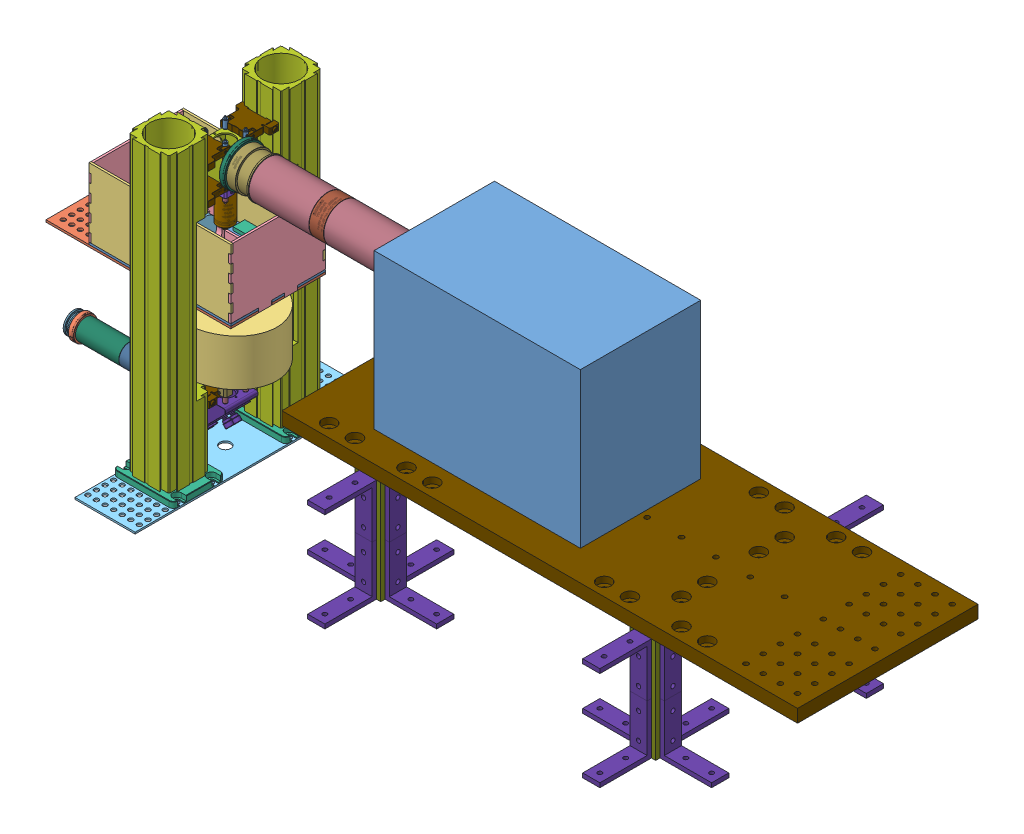
SolidWorks assembly Water Bath DRM, configuration Default. Lengths in mm.
Overall size (1204.68 450.6 419.1).
114 component instances, 38 part files, 41 mates.
Components (placement in the parent):
- WB_0p125_BaseThreaded-1: WB_0p125_BaseThreaded [Default] at (0 3.175 0) size (209.55 3.17 139.7)
- WB_0p125_Base-1: WB_0p125_Base [Default] at origin size (273.05 3.17 139.7)
- WB_0p125_Long-1: WB_0p125_Long [Default] at (0 57.15 -69.85) size (209.55 107.95 3.17)
- WB_0p125_Long-2: WB_0p125_Long [Default] at (0 57.15 66.675) size (209.55 107.95 3.17)
- WB_0p125_Short-1: WB_0p125_Short [Default] at (101.6 57.15 0) x (0 0 1) z (0 1 0) size (139.7 3.17 107.95)
- WB_0p125_Short-2: WB_0p125_Short [Default] at (-104.775 57.15 0) x (0 0 1) z (0 1 0) size (139.7 3.17 107.95)
- Table SubAssembly-1: Table SubAssembly [Default] at (-11.1846 -225.3996 0) x (0 0 -1) z (1 0 0) size (355.6 442.98 89.6)
  - Table-1: Table [Default] at origin size (355.6 2.54 88.9)
  - XT66P1-Solidworks-1: XT66P1-Solidworks [Default] at (-83.0224 2.286 37.592) x (-1 0 0) z (0 0 -1) size (76.2 8.89 89.28)
  - XT66P1-Solidworks-2: XT66P1-Solidworks [Default] at (83.0224 2.286 37.592) size (76.2 8.89 89.28)
  - KCB1-Solidworks-1: KCB1-Solidworks [Default] at (-24.13 99.7796 13.4747) x (0.000001 0 1) z (0 1 0) size (51.13 48.26 51.1) (hidden)
  - RCA1-Solidworks-1: RCA1-Solidworks [Default] at (-24.2926 205.6203 66.0649) x (0 0 -1) z (0 -1 0) size (56.5 73.55 8.89) (hidden)
  - RCA1-Solidworks-2: RCA1-Solidworks [Default] at (24.2926 108.2389 66.0649) x (0 0 -1) z (0 1 0) size (56.5 73.55 8.89) (hidden)
  - XT66-500-modified_v2-1: XT66-500-modified_v2 [Default] at (-83.0224 511.176 37.592) x (0 0 -1) z (0 -1 0) size (66.02 67.06 431.8)
  - XT66-500-modified_v2-2: XT66-500-modified_v2 [Default] at (83.0224 511.176 37.592) x (0 0 1) z (0 -1 0) size (66.02 67.06 431.8)
- Small Condenser Adjustable Sub-Assembly-1: Small Condenser Adjustable Sub-Assembly [Default] at (62.4754 -100.9396 20.3199) x (0 -1 0) z (0 0 1) size (204.14 301.96 127)
  - LB1437-Solidworks-1: LB1437-Solidworks [Default] at (76.2 -223.413 -20.3199) x (0.879994 0 -0.474985) z (0 -1 0) size (25.4 25.4 3.05)
  - LB1761-Solidworks-1: LB1761-Solidworks [Default] at (76.2 -78.613 -20.3199) x (0.962182 0 -0.272406) z (0 -1 0) size (25.4 25.4 8.98)
  - SM1L40-Solidworks-1: SM1L40-Solidworks [Default] at (78.3398 -122.5422 -22.1696) x (-0.992854 0 -0.119336) z (0 1 0) size (30.48 30.48 105.41)
  - CSA1003-Solidworks-1: CSA1003-Solidworks [Default] at (47.6181 -122.449 -34.035) x (0 -1 0) z (0 0 1) size (71.12 13.97 71.12)
  - LCP02-Solidworks-1: LCP02-Solidworks [Default] at (20.32 -35.5599 -20.32) x (0 0 -1) z (1 0 0) size (70.75 70.61 12.7)
  - ER1-Solidworks-1: ER1-Solidworks [Default] at (36.8841 -51.9737 -4.6825) x (0 -0.925141 -0.379624) z (0 -0.379624 0.925141) size (5.99 30.48 5.99)
  - ER1-Solidworks-3: ER1-Solidworks [Default] at (36.8841 -50.6608 -33.7724) x (0 -0.769482 0.638668) z (0 0.638668 0.769482) size (5.99 30.48 5.99)
  - ER1-Solidworks-4: ER1-Solidworks [Default] at (41.8559 -21.5595 -36.5057) x (0 -0.998351 -0.057413) z (0 0.057413 -0.998351) size (5.99 30.48 5.99)
  - SM1T2-Solidworks-1: SM1T2-Solidworks [Default] at (76.2 -248.6152 -20.3199) x (0.998592 0 -0.053039) z (0 1 0) size (31.75 31.75 12.7)
  - SM1L25-Solidworks-1: SM1L25-Solidworks [Default] at (139.9124 -186.275 -15.6668) x (0 -1 0) z (-0.806632 0 -0.591053) size (67.31 30.48 30.48)
  - CP08-Solidworks-3: CP08-Solidworks [Default] at (76.2 -69.215 -20.3199) x (0 0 -1) z (0 1 0) size (41.5 40.64 8.89)
  - KCB1-Solidworks-2: KCB1-Solidworks [Default] at (100.33 -11.43 3.8101) x (-1 0 0) z (0 -1 0) size (51.13 48.26 51.1)
  - ER1-Solidworks-6: ER1-Solidworks [Default] at (36.8841 -20.7263 -3.7781) x (0 -0.795862 0.605478) z (0 0.605478 0.795862) size (5.99 30.48 5.99)
  - RCA2-Solidworks-1: RCA2-Solidworks [Default] at (68.2294 -49.0321 -29.2771) x (0 1 0) z (-1 0 0) size (56.73 41.06 8.89)
  - RCA2-Solidworks-2: RCA2-Solidworks [Default] at (68.2294 -22.0879 -11.3628) x (0 -1 0) z (-1 0 0) size (56.73 41.06 8.89)
  - ER05-Solidworks-1: ER05-Solidworks [Default] at (92.6015 -68.5259 -5.9839) x (0.310188 0 -0.950675) z (0.950675 0 0.310188) size (5.99 17.78 5.99)
  - ER05-Solidworks-2: ER05-Solidworks [Default] at (59.8613 -68.5259 -4.5371) x (-0.22668 0 0.973969) z (-0.973969 0 -0.22668) size (5.99 17.78 5.99)
  - ER05-Solidworks-3: ER05-Solidworks [Default] at (92.2659 -68.5259 -34.1935) size (5.99 17.78 5.99)
  - ER05-Solidworks-4: ER05-Solidworks [Default] at (59.7556 -68.5259 -34.7555) x (-0.375833 0 0.926687) z (-0.926687 0 -0.375833) size (5.99 17.78 5.99)
  - SM1D12D-Solidworks-1: SM1D12D-Solidworks [Default] at (81.3975 -244.783 -22.8892) x (0.973299 0 -0.22954) z (0 1 0) size (35.81 35.81 11.94)
  - SM1D12D-Solidworks-2: SM1D12D-Solidworks [Default] at (70.9424 -73.1298 -22.7639) x (-0.788375 0 -0.615195) z (0 1 0) size (35.81 35.81 11.94)
  - ER1-Solidworks-9: ER1-Solidworks [Default] at (15.1859 -4.2179 -49.5429) x (0 0.95877 -0.284182) z (0 0.284182 0.95877) size (5.99 30.48 5.99)
  - ER1-Solidworks-10: ER1-Solidworks [Default] at (15.1859 -64.6339 -49.076) x (0 0.993069 0.117534) z (0 -0.117534 0.993069) size (5.99 30.48 5.99)
  - ER1-Solidworks-11: ER1-Solidworks [Default] at (15.1859 -4.6008 10.8986) x (0 0.995869 0.090807) z (0 -0.090807 0.995869) size (5.99 30.48 5.99)
  - ER1-Solidworks-12: ER1-Solidworks [Default] at (15.1859 -64.2349 10.4858) x (0 0.96466 -0.263499) z (0 0.263499 0.96466) size (5.99 30.48 5.99)
  - OlympusCondenser-1: OlympusCondenser [Default] at (7.0104 -35.56 -20.3199) x (0 -1 0) z (0 0 -1) size (152.4 107.95 127)
- 500 kHz Tank (21) Opticell-1: 500 kHz Tank (21) Opticell [Default] at (6.35 57.15 0) size (152.4 50.8 50.8)
- 500kHz-1: 500kHz [Default] at (-42.5918 31.75 0) x (1 0 0) z (0 -0.094104 0.995562) size (70.95 43.18 43.18)
- Opticell_Truncated-1: Opticell_Truncated [Default] at (22.5976 32.0671 2.9503) size (53.01 12.75 129.72)
- Objective Sub-Assembly-1: Objective Sub-Assembly [Default] at (61.6077 -289.593 114.3819) x (0 0 -1) z (0 -1 0) size (106.71 57.63 128.02)
  - CM1-DCH-Solidworks-1: CM1-DCH-Solidworks [Web Assembly] at (114.3818 -34.6924 -438.5894) x (0 -1 0) z (0 0 1) size (38.1 45.72 38.1)
  - CP16-Solidworks-1: CP16-Solidworks [Default] at (116.5677 -16.5858 -398.1348) x (0 -1 0) z (0 0 1) size (41.22 40.64 8.89)
  - RCA2-Solidworks-1: RCA2-Solidworks [Default] at (123.339 -21.2203 -499.1988) x (0 -1 0) z (0 0 1) size (56.73 41.06 8.89)
  - RCA2-Solidworks-2: RCA2-Solidworks [Default] at (105.4247 -48.1644 -499.1988) x (0 1 0) z (0 0 1) size (56.73 41.06 8.89)
  - N40X-NIR-Solidworks-1: N40X-NIR-Solidworks [Default] at (114.3819 -34.6923 -375.0894) x (0 0 1) z (0.875921 0.482454 0) size (61.98 27.94 27.94)
  - RCA2-Solidworks-3: RCA2-Solidworks [Default] at (105.4247 -48.1644 -452.2088) x (0 1 0) z (0 0 1) size (56.73 41.06 8.89)
  - RCA2-Solidworks-4: RCA2-Solidworks [Default] at (123.339 -21.2203 -452.2088) x (0 -1 0) z (0 0 1) size (56.73 41.06 8.89)
  - ER1-Solidworks-1: ER1-Solidworks [Default] at (100.293 -20.9473 -404.3535) x (-0.183947 -0.982936 0) z (0.982936 -0.183947 0) size (5.99 30.48 5.99)
  - ER1-Solidworks-2: ER1-Solidworks [Default] at (130.5299 -50.7349 -404.3535) x (0.020475 -0.99979 0) z (0.99979 0.020475 0) size (5.99 30.48 5.99)
  - ER1-Solidworks-3: ER1-Solidworks [Default] at (100.0093 -51.1105 -404.3535) x (-0.386185 -0.922421 0) z (0.922421 -0.386185 0) size (5.99 30.48 5.99)
  - ER1-Solidworks-4: ER1-Solidworks [Default] at (129.6817 -21.2139 -404.3535) x (-0.579753 -0.814792 0) z (0.814792 -0.579753 0) size (5.99 30.48 5.99)
  - ER05-Solidworks-1: ER05-Solidworks [Default] at (129.9725 -48.2584 -461.5035) x (0.933397 0.358845 0) z (-0.358845 0.933397 0) size (5.99 17.78 5.99)
  - ER05-Solidworks-2: ER05-Solidworks [Default] at (97.9162 -50.199 -461.5035) x (-0.886919 0.461926 0) z (-0.461926 -0.886919 0) size (5.99 17.78 5.99)
  - ER05-Solidworks-3: ER05-Solidworks [Default] at (128.9134 -21.1707 -461.5035) x (-0.900043 -0.4358 0) z (0.4358 -0.900043 0) size (5.99 17.78 5.99)
  - ER05-Solidworks-4: ER05-Solidworks [Default] at (100.2773 -18.4261 -461.5035) x (0.989892 0.141823 0) z (-0.141823 0.989892 0) size (5.99 17.78 5.99)
- Camera Sub-Assembly-1: Camera Sub-Assembly [Default] at (36.8213 148.9964 0) x (0 -0.692092 0.721809) z (-1 0 0) size (71.93 71.93 298.88)
  - SM2NFM2-Solidworks-1: SM2NFM2-Solidworks [Default] at (0 0 -285.6832) x (0 1 0) z (-1 0 0) size (63.5 16.37 63.5)
  - TTL200-S8-Solidworks-1: TTL200-S8-Solidworks [Default] at (0 0 -152.5317) size (55.88 55.88 28)
  - SM2V15-Solidworks-1: SM2V15-Solidworks [Default] at (18.0496 -29.8565 -288.422) x (0 0 -1) z (0.951776 0.306793 0) size (51.56 57.15 57.15)
  - SM2M35-Solidworks-1: SM2M35-Solidworks [Default] at (-10.7846 9.351 -219.5042) x (0.99081 -0.135264 0) z (0 0 1) size (55.88 55.88 88.9)
  - SM2M35-Solidworks-2: SM2M35-Solidworks [Default] at (-11.8362 7.9783 -108.9542) x (0.999895 -0.014459 0) z (0 0 1) size (55.88 55.88 88.9)
  - SM2V15-Solidworks-2: SM2V15-Solidworks [Default] at (-9.1968 -33.7176 -16.6413) x (0 0 1) z (-0.999373 0.035397 0) size (51.56 57.15 57.15)
  - SM1T2-Solidworks-1: SM1T2-Solidworks [Default] at (0 0 1.778) x (0.997143 -0.075539 0) z (0 0 1) size (31.75 31.75 12.7)
  - SM2A6-Solidworks-2: SM2A6-Solidworks [Default] at (0 0 -9.144) size (51.69 51.69 5.08)
  - SM2D25D-Solidworks-1: SM2D25D-Solidworks [Default] at (-6.3593 1.1475 -12.9462) x (-1 0 0) z (0 0 -1) size (60.96 60.96 12.32)
- Full Assembly Total Support-1: Full Assembly Total Support [Default] at (624.8382 -22.4536 0) size (762 171.45 419.1)
  - Post SubAssembly-1: Post SubAssembly [Default] at (-254 -152.4 114.3) size (190.5 152.4 190.5)
    - Post-1: Post [Default] at origin size (38.1 152.4 38.1)
    - Hinge-1: Hinge [Default] at (-25.4 6.35 0) x (0 0 -1) z (0 -1 0) size (25.4 76.2 76.2)
    - Hinge-2: Hinge [Default] at (0 6.35 25.4) x (-1 0 0) z (0 -1 0) size (25.4 76.2 76.2)
    - Hinge-3: Hinge [Default] at (25.4 6.35 0) x (0 0 1) z (0 -1 0) size (25.4 76.2 76.2)
    - Hinge-4: Hinge [Default] at (0 6.35 -25.4) x (1 0 0) z (0 -1 0) size (25.4 76.2 76.2)
    - Hinge-5: Hinge [Default] at (25.4 146.05 0) x (0 0 1) z (-1 0 0) size (25.4 76.2 76.2)
    - Hinge-7: Hinge [Default] at (-25.4 146.05 0) x (0 0 -1) z (1 0 0) size (25.4 76.2 76.2)
    - Hinge-8: Hinge [Default] at (0 146.05 25.4) x (-1 0 0) z (0 0 -1) size (25.4 76.2 76.2)
    - Hinge-9: Hinge [Default] at (0 146.05 -25.4) size (25.4 76.2 76.2)
  - Post SubAssembly-2: Post SubAssembly [Default] at (-254 -152.4 -114.3) size (190.5 152.4 190.5)
    - Post-1: Post [Default] at origin size (38.1 152.4 38.1)
    - Hinge-1: Hinge [Default] at (-25.4 6.35 0) x (0 0 -1) z (0 -1 0) size (25.4 76.2 76.2)
    - Hinge-2: Hinge [Default] at (0 6.35 25.4) x (-1 0 0) z (0 -1 0) size (25.4 76.2 76.2)
    - Hinge-3: Hinge [Default] at (25.4 6.35 0) x (0 0 1) z (0 -1 0) size (25.4 76.2 76.2)
    - Hinge-4: Hinge [Default] at (0 6.35 -25.4) x (1 0 0) z (0 -1 0) size (25.4 76.2 76.2)
    - Hinge-5: Hinge [Default] at (25.4 146.05 0) x (0 0 1) z (-1 0 0) size (25.4 76.2 76.2)
    - Hinge-7: Hinge [Default] at (-25.4 146.05 0) x (0 0 -1) z (1 0 0) size (25.4 76.2 76.2)
    - Hinge-8: Hinge [Default] at (0 146.05 25.4) x (-1 0 0) z (0 0 -1) size (25.4 76.2 76.2)
    - Hinge-9: Hinge [Default] at (0 146.05 -25.4) size (25.4 76.2 76.2)
  - Post SubAssembly-3: Post SubAssembly [Default] at (152.4 -152.4 114.3) size (190.5 152.4 190.5)
    - Post-1: Post [Default] at origin size (38.1 152.4 38.1)
    - Hinge-1: Hinge [Default] at (-25.4 6.35 0) x (0 0 -1) z (0 -1 0) size (25.4 76.2 76.2)
    - Hinge-2: Hinge [Default] at (0 6.35 25.4) x (-1 0 0) z (0 -1 0) size (25.4 76.2 76.2)
    - Hinge-3: Hinge [Default] at (25.4 6.35 0) x (0 0 1) z (0 -1 0) size (25.4 76.2 76.2)
    - Hinge-4: Hinge [Default] at (0 6.35 -25.4) x (1 0 0) z (0 -1 0) size (25.4 76.2 76.2)
    - Hinge-5: Hinge [Default] at (25.4 146.05 0) x (0 0 1) z (-1 0 0) size (25.4 76.2 76.2)
    - Hinge-7: Hinge [Default] at (-25.4 146.05 0) x (0 0 -1) z (1 0 0) size (25.4 76.2 76.2)
    - Hinge-8: Hinge [Default] at (0 146.05 25.4) x (-1 0 0) z (0 0 -1) size (25.4 76.2 76.2)
    - Hinge-9: Hinge [Default] at (0 146.05 -25.4) size (25.4 76.2 76.2)
  - Post SubAssembly-4: Post SubAssembly [Default] at (152.4 -152.4 -114.3) size (190.5 152.4 190.5)
    - Post-1: Post [Default] at origin size (38.1 152.4 38.1)
    - Hinge-1: Hinge [Default] at (-25.4 6.35 0) x (0 0 -1) z (0 -1 0) size (25.4 76.2 76.2)
    - Hinge-2: Hinge [Default] at (0 6.35 25.4) x (-1 0 0) z (0 -1 0) size (25.4 76.2 76.2)
    - Hinge-3: Hinge [Default] at (25.4 6.35 0) x (0 0 1) z (0 -1 0) size (25.4 76.2 76.2)
    - Hinge-4: Hinge [Default] at (0 6.35 -25.4) x (1 0 0) z (0 -1 0) size (25.4 76.2 76.2)
    - Hinge-5: Hinge [Default] at (25.4 146.05 0) x (0 0 1) z (-1 0 0) size (25.4 76.2 76.2)
    - Hinge-7: Hinge [Default] at (-25.4 146.05 0) x (0 0 -1) z (1 0 0) size (25.4 76.2 76.2)
    - Hinge-8: Hinge [Default] at (0 146.05 25.4) x (-1 0 0) z (0 0 -1) size (25.4 76.2 76.2)
    - Hinge-9: Hinge [Default] at (0 146.05 -25.4) size (25.4 76.2 76.2)
  - Camera Shelf Full Support v2-1: Camera Shelf Full Support v2 [Default] at origin size (762 19.05 266.7)
- hpvx2-1: hpvx2 [Default] at (488.0998 -3.4036 0) size (311.15 228.6 177.8)
Mates (geometry in assembly coordinates):
- Coincident1: coincident aligned: plane of WB_0p125_BaseThreaded-1 through (-101.6 6.35 66.675) normal (0 0 1); plane of WB_0p125_Base-1 through (-101.6 3.175 66.675) normal (0 0 1)
- Coincident2: coincident aligned: plane of WB_0p125_BaseThreaded-1 through (101.6 6.35 66.675) normal (1 0 0); plane of WB_0p125_Base-1 through (101.6 3.175 66.675) normal (1 0 0)
- Coincident3: coincident anti-aligned: plane of WB_0p125_BaseThreaded-1 through (0 3.175 0) normal (0 -1 0); plane of WB_0p125_Base-1 through (0 3.175 0) normal (0 1 0)
- Coincident4: coordinate: point of WB_0p125_Base-1; point of assembly
- Coincident5: coincident aligned: plane of WB_0p125_BaseThreaded-1 through (101.6 6.35 66.675) normal (1 0 0); plane of WB_0p125_Long-2 through (101.6 6.35 69.85) normal (1 0 0)
- Coincident6: coincident anti-aligned: plane of WB_0p125_BaseThreaded-1 through (0 6.35 0) normal (0 1 0); plane of WB_0p125_Long-2 through (-101.6 6.35 69.85) normal (0 -1 0)
- Coincident8: coincident anti-aligned: plane of WB_0p125_BaseThreaded-1 through (0 6.35 0) normal (0 1 0); plane of WB_0p125_Long-1 through (-101.6 6.35 -66.675) normal (0 -1 0)
- Coincident9: coincident aligned: plane of WB_0p125_BaseThreaded-1 through (-101.6 6.35 66.675) normal (-1 0 0); plane of WB_0p125_Long-1 through (-101.6 6.35 -66.675) normal (-1 0 0)
- Coincident11: coincident anti-aligned: plane of WB_0p125_BaseThreaded-1 through (-101.6 6.35 66.675) normal (-1 0 0); plane of WB_0p125_Short-2 through (-101.6 57.15 0) normal (1 0 0)
- Coincident12: coincident anti-aligned: plane of WB_0p125_BaseThreaded-1 through (0 6.35 0) normal (0 1 0); plane of WB_0p125_Short-2 through (-101.6 6.35 -66.675) normal (0 -1 0)
- Coincident14: coincident anti-aligned: plane of WB_0p125_Long-2 through (0 57.15 66.675) normal (0 0 -1); plane of WB_0p125_Short-2 through (-101.6 107.95 66.675) normal (0 0 1)
- Coincident16: coincident anti-aligned: plane of WB_0p125_Long-2 through (0 57.15 66.675) normal (0 0 -1); plane of WB_0p125_Short-1 through (104.775 107.95 66.675) normal (0 0 1)
- Coincident18: coincident anti-aligned: plane of WB_0p125_Long-1 through (0 57.15 -66.675) normal (0 0 1); plane of WB_0p125_Short-2 through (-101.6 107.95 -66.675) normal (0 0 -1)
- Coincident19: coincident anti-aligned: plane of WB_0p125_BaseThreaded-1 through (-101.6 6.35 -66.675) normal (0 0 -1); plane of WB_0p125_Long-1 through (0 57.15 -66.675) normal (0 0 1)
- Coincident20: coincident aligned: plane of WB_0p125_Long-2 through (104.775 107.95 66.675) normal (1 0 0); plane of WB_0p125_Short-1 through (104.775 57.15 0) normal (1 0 0)
- Coincident21: coincident aligned: plane of WB_0p125_Base-1 through (0 0 0) normal (0 -1 0); plane of WB_0p125_Short-1 through (104.775 0 9.525) normal (0 -1 0)
- Coincident28: coincident anti-aligned: plane of Table SubAssembly-1/Table-1 through (-11.1846 -225.3996 0) normal (0 0 -1); plane of assembly through (0 0 0) normal (0 0 1)
- Concentric7: concentric aligned: circle of Table SubAssembly-1/Table-1; circle of Small Condenser Adjustable Sub-Assembly-1/OlympusCondenser-1
- Parallel1: parallel aligned: plane of Table SubAssembly-1/XT66-500-modified_v2-1 through (6.0694 -214.2236 116.5515) normal (0 0 1); plane of Small Condenser Adjustable Sub-Assembly-1/CSA1003-Solidworks-1 through (62.4754 -100.9396 35.56) normal (0 0 1)
- Concentric8: concentric aligned: circle of WB_0p125_BaseThreaded-1; circle of 500 kHz Tank (21) Opticell-1
- Concentric10: concentric aligned: circle of WB_0p125_BaseThreaded-1; circle of 500 kHz Tank (21) Opticell-1
- Coincident29: coincident anti-aligned: plane of WB_0p125_BaseThreaded-1 through (0 6.35 0) normal (0 1 0); plane of 500 kHz Tank (21) Opticell-1 through (-69.85 6.35 25.4) normal (0 -1 0)
- Concentric11: concentric aligned: cylinder of 500 kHz Tank (21) Opticell-1 through (-146.1329 31.75 0) axis (-1 0 0) radius 22.225; cylinder of 500kHz-1 through (-42.5918 31.75 0) axis (-1 0 0) radius 21.59
- Coincident30: coincident anti-aligned: plane of 500 kHz Tank (21) Opticell-1 through (-4.9109 53.975 0) normal (-1 0 0); plane of 500kHz-1 through (-4.9109 53.2442 2.0317) normal (1 0 0)
- Coincident31: coincident anti-aligned: plane of 500 kHz Tank (21) Opticell-1 through (6.35 25.6921 0) normal (0 1 0); plane of Opticell_Truncated-1 through (22.5976 25.6921 2.9503) normal (0 -1 0)
- Coincident32: coincident anti-aligned: plane of 500 kHz Tank (21) Opticell-1 through (58.6526 25.6921 -25.4) normal (-1 0 0); plane of Opticell_Truncated-1 through (58.6526 34.5671 51.6503) normal (1 0 0)
- Coincident33: coincident anti-aligned: plane of WB_0p125_Base-1 through (0 0 0) normal (0 -1 0); plane of Small Condenser Adjustable Sub-Assembly-1/OlympusCondenser-1 through (26.9154 0 0) normal (0 1 0)
- Distance1: distance = 25.4 mm anti-aligned: plane of Small Condenser Adjustable Sub-Assembly-1/CP08-Solidworks-3 through (-2.2946 -197.4596 18.034) normal (0 -1 0); plane of Table SubAssembly-1/Table-1 through (-11.1846 -222.8596 0) normal (0 1 0)
- Concentric12: concentric aligned: circle of Table SubAssembly-1/Table-1; circle of Objective Sub-Assembly-1/N40X-NIR-Solidworks-1
- Parallel2: parallel aligned: plane of Table SubAssembly-1/XT66-500-modified_v2-2 through (59.4152 -214.2236 -103.3604) normal (1 0 0); plane of Objective Sub-Assembly-1/CM1-DCH-Solidworks-1 through (45.9653 129.9464 -19.05) normal (1 0 0)
- Concentric13: concentric aligned: circle of Objective Sub-Assembly-1/CM1-DCH-Solidworks-1; cylinder of Camera Sub-Assembly-1/SM2M35-Solidworks-2 through (136.618 148.9964 0) axis (-1 0 0) radius 27.94
- Distance2: distance = 40.64 mm aligned: plane of Table SubAssembly-1/XT66-500-modified_v2-2 through (-6.6004 217.5764 -49.4934) normal (0 1 0); plane of Objective Sub-Assembly-1/RCA2-Solidworks-1 through (45.9653 176.9364 -13.6187) normal (0 1 0)
- Coincident36: coincident anti-aligned: plane of Objective Sub-Assembly-1/CM1-DCH-Solidworks-1 through (45.9653 129.9464 -19.05) normal (1 0 0); plane of Camera Sub-Assembly-1/SM2A6-Solidworks-2 through (45.9653 158.4842 9.0972) normal (-1 0 0)
- Concentric14: concentric anti-aligned: cylinder of Camera Sub-Assembly-1/SM2M35-Solidworks-1 through (247.168 148.9964 0) axis (-1 0 0) radius 27.94; cylinder of hpvx2-1 through (335.6998 148.9964 0) axis (1 0 0) radius 29.1375
- Coincident37: coincident anti-aligned: plane of Camera Sub-Assembly-1/SM2NFM2-Solidworks-1 through (329.3498 149.0478 0.0494) normal (1 0 0); plane of hpvx2-1 through (329.3498 148.9964 0) normal (-1 0 0)
- Parallel3: parallel aligned: plane of Table SubAssembly-1/XT66-500-modified_v2-1 through (59.4152 217.5764 49.4934) normal (0 1 0); plane of hpvx2-1 through (488.0998 225.1964 0) normal (0 1 0)
- Distance3: distance = 98.1746 mm aligned: plane of WB_0p125_Short-2 through (-104.775 57.15 0) normal (-1 0 0); plane of Table SubAssembly-1/XT66-500-modified_v2-1 through (-6.6004 -214.2236 103.3604) normal (-1 0 0)
- Coincident38: coincident anti-aligned: plane of Full Assembly Total Support-1/Camera Shelf Full Support v2-1 through (624.8382 -3.4036 0) normal (0 1 0); plane of hpvx2-1 through (488.0998 -3.4036 0) normal (0 -1 0)
- Parallel4: parallel aligned: plane of Full Assembly Total Support-1/Camera Shelf Full Support v2-1 through (1005.8382 -3.4036 133.35) normal (1 0 0); plane of hpvx2-1 through (640.4998 225.1964 88.9) normal (1 0 0)
- Parallel5: parallel aligned: plane of Full Assembly Total Support-1/Camera Shelf Full Support v2-1 through (243.8382 -3.4036 -133.35) normal (0 0 -1); plane of hpvx2-1 through (335.6998 225.1964 -88.9) normal (0 0 -1)
- Coincident39: coincident aligned: plane of Full Assembly Total Support-1/Camera Shelf Full Support v2-1 through (624.8382 -22.4536 0) normal (0 0 1); plane of hpvx2-1 through (488.0998 -3.4036 0) normal (0 0 1)
